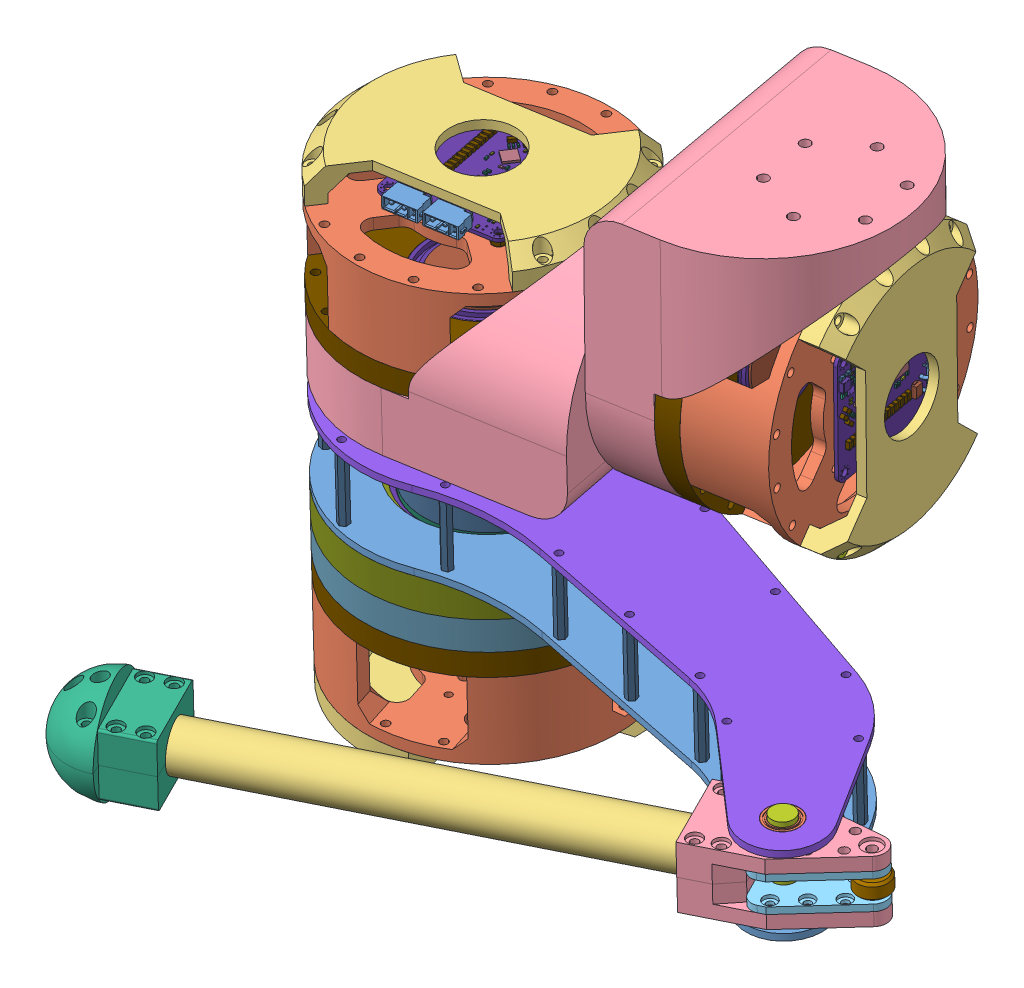
SolidWorks assembly leg, configuration Default. Lengths in mm. (continued)
Components (placement in the parent): (continued)
- Cycloidal _v3-1: Cycloidal _v3 [Default] at (95.6254 359.4899 346.7984) x (0.586151 0.024345 -0.809836) z (-0.810184 0.024334 -0.585671) size (173.36 87.57 173.15) (continued)
  - m13_bearing-34: m13_bearing [Default] at (13.4541 98.1947 126.1847) x (0.227678 0.000091 0.973736) z (0.973736 0.000388 -0.227678) size (13 16 13) (continued)
    - radial ball bearing_68_iso-1: radial ball bearing_68_iso [ISO 15 RBB - 286 - 10,SI,NC,10_68] at (8.4921 16.0508 14.8914) x (0 1 0) z (0 0 1) size (5 13 13)
    - radial ball bearing_68_iso-2: radial ball bearing_68_iso [ISO 15 RBB - 286 - 10,SI,NC,10_68] at (8.4921 11.0508 14.8914) x (0 1 0) z (0 0 1) size (5 13 13)
  - m13_bearing-35: m13_bearing [Default] at (-1.0662 98.1889 116.3132) x (0.227678 0.000091 0.973736) z (0.973736 0.000388 -0.227678) size (13 16 13)
    - m6-1: m6 [Default] at (8.4921 2.5508 14.8914) size (6 16 6)
    - radial ball bearing_68_iso-1: radial ball bearing_68_iso [ISO 15 RBB - 286 - 10,SI,NC,10_68] at (8.4921 16.0508 14.8914) x (0 1 0) z (0 0 1) size (5 13 13)
    - radial ball bearing_68_iso-2: radial ball bearing_68_iso [ISO 15 RBB - 286 - 10,SI,NC,10_68] at (8.4921 11.0508 14.8914) x (0 1 0) z (0 0 1) size (5 13 13)
  - m13_bearing-36: m13_bearing [Default] at (-10.7036 98.185 101.6364) x (0.227678 0.000091 0.973736) z (0.973736 0.000388 -0.227678) size (13 16 13)
    - m6-1: m6 [Default] at (8.4921 2.5508 14.8914) size (6 16 6)
    - radial ball bearing_68_iso-1: radial ball bearing_68_iso [ISO 15 RBB - 286 - 10,SI,NC,10_68] at (8.4921 16.0508 14.8914) x (0 1 0) z (0 0 1) size (5 13 13)
    - radial ball bearing_68_iso-2: radial ball bearing_68_iso [ISO 15 RBB - 286 - 10,SI,NC,10_68] at (8.4921 11.0508 14.8914) x (0 1 0) z (0 0 1) size (5 13 13)
  - m13_bearing-1: m13_bearing [Default] at (-0.4494 98.1891 62.778) x (0.736525 0.000294 0.676411) z (0.676411 0.00027 -0.736525) size (13 16 13)
    - m6-1: m6 [Default] at (8.4921 2.5508 14.8914) size (6 16 6)
    - radial ball bearing_68_iso-1: radial ball bearing_68_iso [ISO 15 RBB - 286 - 10,SI,NC,10_68] at (8.4921 16.0508 14.8914) x (0 1 0) z (0 0 1) size (5 13 13)
    - radial ball bearing_68_iso-2: radial ball bearing_68_iso [ISO 15 RBB - 286 - 10,SI,NC,10_68] at (8.4921 11.0508 14.8914) x (0 1 0) z (0 0 1) size (5 13 13)
  - m13_bearing-2: m13_bearing [Default] at (48.5236 98.2087 124.7001) x (0.120271 0.000048 0.992741) z (0.992741 0.000396 -0.120271) size (13 16 13)
    - m6-1: m6 [Default] at (8.4921 2.5508 14.8914) size (6 16 6)
    - radial ball bearing_68_iso-1: radial ball bearing_68_iso [ISO 15 RBB - 286 - 10,SI,NC,10_68] at (8.4921 16.0508 14.8914) x (0 1 0) z (0 0 1) size (5 13 13)
    - radial ball bearing_68_iso-2: radial ball bearing_68_iso [ISO 15 RBB - 286 - 10,SI,NC,10_68] at (8.4921 11.0508 14.8914) x (0 1 0) z (0 0 1) size (5 13 13)
  - m13_bearing-3: m13_bearing [Default] at (32.5019 98.2023 52.3604) x (0.833889 0.000333 0.551933) z (0.551932 0.00022 -0.833889) size (13 16 13)
    - m6-1: m6 [Default] at (8.4921 2.5508 14.8914) size (6 16 6)
    - radial ball bearing_68_iso-1: radial ball bearing_68_iso [ISO 15 RBB - 286 - 10,SI,NC,10_68] at (8.4921 16.0508 14.8914) x (0 1 0) z (0 0 1) size (5 13 13)
    - radial ball bearing_68_iso-2: radial ball bearing_68_iso [ISO 15 RBB - 286 - 10,SI,NC,10_68] at (8.4921 11.0508 14.8914) x (0 1 0) z (0 0 1) size (5 13 13)
  - m13_bearing-4: m13_bearing [Default] at (77.3632 98.2202 81.8307) x (0.022268 0.000009 0.999752) z (0.999752 0.000399 -0.022268) size (13 16 13)
    - m6-1: m6 [Default] at (8.4921 2.5508 14.8914) size (6 16 6)
    - radial ball bearing_68_iso-1: radial ball bearing_68_iso [ISO 15 RBB - 286 - 10,SI,NC,10_68] at (8.4921 16.0508 14.8914) x (0 1 0) z (0 0 1) size (5 13 13)
    - radial ball bearing_68_iso-2: radial ball bearing_68_iso [ISO 15 RBB - 286 - 10,SI,NC,10_68] at (8.4921 11.0508 14.8914) x (0 1 0) z (0 0 1) size (5 13 13)
  - m13_bearing-5: m13_bearing [Default] at (73.5091 98.2186 99.5852) x (0.059133 0.000024 0.99825) z (0.99825 0.000398 -0.059133) size (13 16 13)
    - m6-1: m6 [Default] at (8.4921 2.5508 14.8914) size (6 16 6)
    - radial ball bearing_68_iso-1: radial ball bearing_68_iso [ISO 15 RBB - 286 - 10,SI,NC,10_68] at (8.4921 16.0508 14.8914) x (0 1 0) z (0 0 1) size (5 13 13)
    - radial ball bearing_68_iso-2: radial ball bearing_68_iso [ISO 15 RBB - 286 - 10,SI,NC,10_68] at (8.4921 11.0508 14.8914) x (0 1 0) z (0 0 1) size (5 13 13)
  - m13_bearing-6: m13_bearing [Default] at (13.4333 98.1947 47.0643) x (0.451561 0.00018 0.89224) z (0.89224 0.000356 -0.451561) size (13 16 13)
    - m6-1: m6 [Default] at (8.4921 2.5508 14.8914) size (6 16 6)
    - radial ball bearing_68_iso-1: radial ball bearing_68_iso [ISO 15 RBB - 286 - 10,SI,NC,10_68] at (8.4921 16.0508 14.8914) x (0 1 0) z (0 0 1) size (5 13 13)
    - radial ball bearing_68_iso-2: radial ball bearing_68_iso [ISO 15 RBB - 286 - 10,SI,NC,10_68] at (8.4921 11.0508 14.8914) x (0 1 0) z (0 0 1) size (5 13 13)
  - m13_bearing-7: m13_bearing [Default] at (57.1526 98.2121 32.9496) x (-0.545813 -0.000218 0.837907) z (0.837907 0.000334 0.545813) size (13 16 13)
    - m6-1: m6 [Default] at (8.4921 2.5508 14.8914) size (6 16 6)
    - radial ball bearing_68_iso-1: radial ball bearing_68_iso [ISO 15 RBB - 286 - 10,SI,NC,10_68] at (8.4921 16.0508 14.8914) x (0 1 0) z (0 0 1) size (5 13 13)
    - radial ball bearing_68_iso-2: radial ball bearing_68_iso [ISO 15 RBB - 286 - 10,SI,NC,10_68] at (8.4921 11.0508 14.8914) x (0 1 0) z (0 0 1) size (5 13 13)
  - m13_bearing-8: m13_bearing [Default] at (73.1034 98.2185 66.7178) x (0.158553 0.000063 0.98735) z (0.98735 0.000394 -0.158553) size (13 16 13)
    - m6-1: m6 [Default] at (8.4921 2.5508 14.8914) size (6 16 6)
    - radial ball bearing_68_iso-1: radial ball bearing_68_iso [ISO 15 RBB - 286 - 10,SI,NC,10_68] at (8.4921 16.0508 14.8914) x (0 1 0) z (0 0 1) size (5 13 13)
    - radial ball bearing_68_iso-2: radial ball bearing_68_iso [ISO 15 RBB - 286 - 10,SI,NC,10_68] at (8.4921 11.0508 14.8914) x (0 1 0) z (0 0 1) size (5 13 13)
  - m13_bearing-9: m13_bearing [Default] at (74.5316 98.219 41.6624) x (-0.687134 -0.000274 0.72653) z (0.72653 0.00029 0.687134) size (13 16 13)
    - m6-1: m6 [Default] at (8.4921 2.5508 14.8914) size (6 16 6)
    - radial ball bearing_68_iso-1: radial ball bearing_68_iso [ISO 15 RBB - 286 - 10,SI,NC,10_68] at (8.4921 16.0508 14.8914) x (0 1 0) z (0 0 1) size (5 13 13)
    - radial ball bearing_68_iso-2: radial ball bearing_68_iso [ISO 15 RBB - 286 - 10,SI,NC,10_68] at (8.4921 11.0508 14.8914) x (0 1 0) z (0 0 1) size (5 13 13)
  - m13_bearing-11: m13_bearing [Default] at (30.0113 98.2013 136.2104) x (0.57351 0.000229 0.819198) z (0.819198 0.000327 -0.57351) size (13 16 13)
    - m6-1: m6 [Default] at (8.4921 2.5508 14.8914) size (6 16 6)
    - radial ball bearing_68_iso-1: radial ball bearing_68_iso [ISO 15 RBB - 286 - 10,SI,NC,10_68] at (8.4921 16.0508 14.8914) x (0 1 0) z (0 0 1) size (5 13 13)
    - radial ball bearing_68_iso-2: radial ball bearing_68_iso [ISO 15 RBB - 286 - 10,SI,NC,10_68] at (8.4921 11.0508 14.8914) x (0 1 0) z (0 0 1) size (5 13 13)
  - m13_bearing-12: m13_bearing [Default] at (62.5932 98.2143 116.7506) x (0.22335 0.000089 0.974738) z (0.974738 0.000389 -0.22335) size (13 16 13)
    - m6-1: m6 [Default] at (8.4921 2.5508 14.8914) size (6 16 6)
    - radial ball bearing_68_iso-1: radial ball bearing_68_iso [ISO 15 RBB - 286 - 10,SI,NC,10_68] at (8.4921 16.0508 14.8914) x (0 1 0) z (0 0 1) size (5 13 13)
    - radial ball bearing_68_iso-2: radial ball bearing_68_iso [ISO 15 RBB - 286 - 10,SI,NC,10_68] at (8.4921 11.0508 14.8914) x (0 1 0) z (0 0 1) size (5 13 13)
  - M3x4x4.2_brass_insert-22: M3x4x4.2_brass_insert [Default] at (43.4837 68.6558 90.1203) x (0.984609 0.000393 -0.174769) z (0.174769 0.00007 0.984609) size (4 4 4)
  - M3x4x4.2_brass_insert-23: M3x4x4.2_brass_insert [Default] at (51.4229 68.659 89.1361) x (0.984609 0.000393 -0.174769) z (0.174769 0.00007 0.984609) size (4 4 4)
  - radial ball bearing_68_iso-44: radial ball bearing_68_iso [ISO 15 RBB - 1715 - 26,SI,NC,26_68] at (47.2636 81.6573 88.1396) x (0.000399 -1 0) z (0.171535 0.000068 0.985178) size (4 21 21)
  - radial ball bearing_68_iso-45: radial ball bearing_68_iso [ISO 15 RBB - 1715 - 26,SI,NC,26_68] at (47.4429 94.6574 89.6282) x (0.000399 -1 0) z (0.819169 0.000327 0.573552) size (4 21 21)
  - radial ball bearing_68_iso-46: radial ball bearing_68_iso [ISO 15 RBB - 1715 - 26,SI,NC,26_68] at (47.6295 89.6575 91.1168) x (-0.000399 1 0) z (0 0 1) size (4 21 21)
  - foc-motor-controller.step-1: foc-motor-controller.step [Default] at (47.4677 32.6574 89.6282) x (0.701413 0.00028 0.712755) z (0.000399 -1 0) size (57.23 50 8.13)
    - RTA0040B.step-1: RTA0040B.step [Default] at (12.5014 -1.6986 1.595) x (-0.707107 -0.707107 0) z (0 0 1) size (6 6 1)
      - FRAME.step-1: FRAME.step [Default] x (1 0 0) z (0 -1 0) size (6 0.2 6)
        - SOLID.step-1: SOLID.step [Default] at origin size (0.4 0.2 0.22)
        - SOLID-0.step-1: SOLID-0.step [Default] at origin size (0.4 0.2 0.22)
        - SOLID-1.step-1: SOLID-1.step [Default] at origin size (0.4 0.2 0.22)
        - SOLID-2.step-1: SOLID-2.step [Default] at origin size (0.4 0.2 0.22)
        - SOLID-3.step-1: SOLID-3.step [Default] at origin size (0.4 0.2 0.22)
        - SOLID-4.step-1: SOLID-4.step [Default] at origin size (0.4 0.2 0.22)
        - SOLID-5.step-1: SOLID-5.step [Default] at origin size (0.4 0.2 0.22)
        - SOLID-6.step-1: SOLID-6.step [Default] at origin size (0.4 0.2 0.22)
        - SOLID-7.step-1: SOLID-7.step [Default] at origin size (0.4 0.2 0.22)
        - SOLID-8.step-1: SOLID-8.step [Default] at origin size (0.4 0.2 0.22)
        - SOLID-9.step-1: SOLID-9.step [Default] at origin size (0.22 0.2 0.4)
        - SOLID-10.step-1: SOLID-10.step [Default] at origin size (0.22 0.2 0.4)
        - SOLID-11.step-1: SOLID-11.step [Default] at origin size (0.22 0.2 0.4)
        - SOLID-12.step-1: SOLID-12.step [Default] at origin size (0.22 0.2 0.4)
        - SOLID-13.step-1: SOLID-13.step [Default] at origin size (0.22 0.2 0.4)
        - SOLID-14.step-1: SOLID-14.step [Default] at origin size (0.22 0.2 0.4)
        - SOLID-15.step-1: SOLID-15.step [Default] at origin size (0.22 0.2 0.4)
        - SOLID-16.step-1: SOLID-16.step [Default] at origin size (0.22 0.2 0.4)
        - SOLID-17.step-1: SOLID-17.step [Default] at origin size (4.15 0.2 4.15)
        - SOLID-18.step-1: SOLID-18.step [Default] at origin size (0.28 0.1 0.28)
        - SOLID-19.step-1: SOLID-19.step [Default] at origin size (0.28 0.1 0.28)
        - SOLID-20.step-1: SOLID-20.step [Default] at origin size (0.28 0.1 0.28)
        - SOLID-21.step-1: SOLID-21.step [Default] at origin size (0.28 0.1 0.28)
        - SOLID-22.step-1: SOLID-22.step [Default] at origin size (0.4 0.2 0.22)
        - SOLID-23.step-1: SOLID-23.step [Default] at origin size (0.4 0.2 0.22)
        - SOLID-24.step-1: SOLID-24.step [Default] at origin size (0.4 0.2 0.22)
        - SOLID-25.step-1: SOLID-25.step [Default] at origin size (0.4 0.2 0.22)
        - SOLID-26.step-1: SOLID-26.step [Default] at origin size (0.4 0.2 0.22)
        - SOLID-27.step-1: SOLID-27.step [Default] at origin size (0.4 0.2 0.22)
        - SOLID-28.step-1: SOLID-28.step [Default] at origin size (0.4 0.2 0.22)
        - SOLID-29.step-1: SOLID-29.step [Default] at origin size (0.4 0.2 0.22)
        - SOLID-30.step-1: SOLID-30.step [Default] at origin size (0.4 0.2 0.22)
        - SOLID-31.step-1: SOLID-31.step [Default] at origin size (0.4 0.2 0.22)
        - SOLID-32.step-1: SOLID-32.step [Default] at origin size (0.22 0.2 0.4)
        - SOLID-33.step-1: SOLID-33.step [Default] at origin size (0.22 0.2 0.4)
        - SOLID-34.step-1: SOLID-34.step [Default] at origin size (0.22 0.2 0.4)
        - SOLID-35.step-1: SOLID-35.step [Default] at origin size (0.22 0.2 0.4)
        - SOLID-36.step-1: SOLID-36.step [Default] at origin size (0.22 0.2 0.4)
        - SOLID-37.step-1: SOLID-37.step [Default] at origin size (0.22 0.2 0.4)
        - SOLID-38.step-1: SOLID-38.step [Default] at origin size (0.22 0.2 0.4)
        - SOLID-39.step-1: SOLID-39.step [Default] at origin size (0.22 0.2 0.4)
        - SOLID-40.step-1: SOLID-40.step [Default] at origin size (0.22 0.2 0.4)
        - SOLID-41.step-1: SOLID-41.step [Default] at origin size (0.22 0.2 0.4)
        - SOLID-42.step-1: SOLID-42.step [Default] at origin size (0.22 0.2 0.4)
        - SOLID-43.step-1: SOLID-43.step [Default] at origin size (0.22 0.2 0.4)
      - BODY.step-1: BODY.step [Default] at (0 0 0.025) x (1 0 0) z (0 -1 0) size (6 0.97 6)
    - Resonator_SMD_Murata_CSTxExxV-3Pin_3.0x1.1mm.step-1: Resonator_SMD_Murata_CSTxExxV-3Pin_3.0x1.1mm.step [Default] at (1.8 -7 1.595) x (0 1 0) z (0 0 1) size (3.2 1.35 0.9)
    - C_0603_1608Metric.step-1: C_0603_1608Metric.step [Default] at (6.2 -16.8 1.595) x (0 -1 0) z (0 0 1) size (1.6 0.8 0.8)
    - R_0603_1608Metric.step-1: R_0603_1608Metric.step [Default] at (11.8 -7.375 1.595) x (0 1 0) z (0 0 1) size (1.6 0.8 0.45)
    - R_0603_1608Metric.step-2: R_0603_1608Metric.step [Default] at (13.8 -16.8 1.595) x (0 1 0) z (0 0 1) size (1.6 0.8 0.45)
    - R_0603_1608Metric.step-3: R_0603_1608Metric.step [Default] at (18.1 -5.36 1.595) size (1.6 0.8 0.45)
    - C_0603_1608Metric.step-2: C_0603_1608Metric.step [Default] at (2.6 -0.5 1.595) x (0 -1 0) z (0 0 1) size (1.6 0.8 0.8)
    - R_0603_1608Metric.step-4: R_0603_1608Metric.step [Default] at (14.6 -11.3 1.595) x (0 1 0) z (0 0 1) size (1.6 0.8 0.45)
    - L_APV_ANR4020.step-1: L_APV_ANR4020.step [Default] at (22.3 -13.7 1.595) x (0 -1 0) z (0 0 1) size (4.02 4 2)
    - C_0603_1608Metric.step-3: C_0603_1608Metric.step [Default] at (0.3 -12.6 1.595) x (-1 0 0) z (0 0 1) size (1.6 0.8 0.8)
    - C_1206_3216Metric.step-1: C_1206_3216Metric.step [Default] at (15.7 11 1.595) x (0 1 0) z (0 0 1) size (3.2 1.6 1.6)
    - C_0603_1608Metric.step-4: C_0603_1608Metric.step [Default] at (0.3 -9.6 1.595) size (1.6 0.8 0.8)
    - R_0603_1608Metric.step-5: R_0603_1608Metric.step [Default] at (12.3 -16.8 1.595) x (0 1 0) z (0 0 1) size (1.6 0.8 0.45)
    - C_0603_1608Metric.step-5: C_0603_1608Metric.step [Default] at (-0.3 -16.6 1.595) x (0 1 0) z (0 0 1) size (1.6 0.8 0.8)
    - R_0603_1608Metric.step-6: R_0603_1608Metric.step [Default] at (10.9 4.1 1.595) size (1.6 0.8 0.45)
    - C_1206_3216Metric.step-2: C_1206_3216Metric.step [Default] at (6.3 11 1.595) x (0 1 0) z (0 0 1) size (3.2 1.6 1.6)
    - XT30PW_2_2_-M.G.B.step-1: XT30PW_2_2_-M.G.B.step [Default] at (-20.5 9.5 1.595) x (0 -1 0) z (-1 0 0) size (15.5 7.1 12.53)
    - R_0603_1608Metric.step-7: R_0603_1608Metric.step [Default] at (0.3 -11.1 1.595) size (1.6 0.8 0.45)
    - C_0603_1608Metric.step-6: C_0603_1608Metric.step [Default] at (19 -0.4 1.595) x (-0.707107 -0.707107 0) z (0 0 1) size (1.6 0.8 0.8)
    - C_1206_3216Metric.step-3: C_1206_3216Metric.step [Default] at (13.3 11 1.595) x (0 1 0) z (0 0 1) size (3.2 1.6 1.6)
    - R_0603_1608Metric.step-8: R_0603_1608Metric.step [Default] at (10.2 -7.375 1.595) x (0 -1 0) z (0 0 1) size (1.6 0.8 0.45)
    - JST_GH_SM08B-GHS-TB_1x08-1MP_P1.25mm_Horizontal.step-1: JST_GH_SM08B-GHS-TB_1x08-1MP_P1.25mm_Horizontal.step [Default] at (10 -22 1.595) size (13.25 4.95 4.25)
    - C_1206_3216Metric.step-4: C_1206_3216Metric.step [Default] at (-12.3 11 1.595) x (0 1 0) z (0 0 1) size (3.2 1.6 1.6)
    - JST_GH_SM06B-GHS-TB_1x06-1MP_P1.25mm_Horizontal.step-1: JST_GH_SM06B-GHS-TB_1x06-1MP_P1.25mm_Horizontal.step [Default] at (-4.3 -22 1.595) size (10.75 4.95 4.25)
    - C_0603_1608Metric.step-7: C_0603_1608Metric.step [Default] at (7.3 -4.5 1.595) x (-1 0 0) z (0 0 1) size (1.6 0.8 0.8)
    - R_0603_1608Metric.step-9: R_0603_1608Metric.step [Default] at (18.1 -3.86 1.595) x (-1 0 0) z (0 0 1) size (1.6 0.8 0.45)
    - C_1206_3216Metric.step-5: C_1206_3216Metric.step [Default] at (22.6794 -1.2206 1.595) x (0.707107 -0.707107 0) z (0 0 1) size (3.2 1.6 1.6)
    - R_Array_Convex_4x0402.step-1: R_Array_Convex_4x0402.step [Default] at (6.8 -2.5 1.595) size (1 2 0.35)
    - R_0603_1608Metric.step-10: R_0603_1608Metric.step [Default] at (7.7 -16.8 1.595) x (0 -1 0) z (0 0 1) size (1.6 0.8 0.45)
    - C_1206_3216Metric.step-6: C_1206_3216Metric.step [Default] at (8.7 11 1.595) x (0 1 0) z (0 0 1) size (3.2 1.6 1.6)
    - C_0603_1608Metric.step-8: C_0603_1608Metric.step [Default] at (16.1 -11.3 1.595) x (0 1 0) z (0 0 1) size (1.6 0.8 0.8)
    - SOT-23-5.step-1: SOT-23-5.step [Default] at (-3.1 -16.6 1.595) x (-1 0 0) z (0 0 1) size (2.8 2.9 1.55)
    - C_0603_1608Metric.step-9: C_0603_1608Metric.step [Default] at (17.8 -13.6 1.595) size (1.6 0.8 0.8)
    - R_0603_1608Metric.step-11: R_0603_1608Metric.step [Default] at (-11.5 -20.3875 1.595) x (0 -1 0) z (0 0 1) size (1.6 0.8 0.45)
    - C_0603_1608Metric.step-10: C_0603_1608Metric.step [Default] at (-12.4 2.3 1.595) x (0 1 0) z (0 0 1) size (1.6 0.8 0.8)
    - C_1206_3216Metric.step-7: C_1206_3216Metric.step [Default] at (18 11 1.595) x (0 1 0) z (0 0 1) size (3.2 1.6 1.6)
    - R_0603_1608Metric.step-12: R_0603_1608Metric.step [Default] at (-10.8105 -14.9971 1.595) x (-1 0 0) z (0 0 1) size (1.6 0.8 0.45)
    - C_0603_1608Metric.step-11: C_0603_1608Metric.step [Default] at (-13.8 -9.4 1.595) x (-1 0 0) z (0 0 1) size (1.6 0.8 0.8)
    - R_0603_1608Metric.step-13: R_0603_1608Metric.step [Default] at (-23.15 -14.5 1.595) x (-1 0 0) z (0 0 1) size (1.6 0.8 0.45)
    - C_0603_1608Metric.step-12: C_0603_1608Metric.step [Default] at (1.1 -0.2 1.595) x (0 1 0) z (0 0 1) size (1.6 0.8 0.8)
    - D_0805_2012Metric.step-1: D_0805_2012Metric.step [Default] at (22.9 -9.6 1.595) x (0 1 0) z (0 0 1) size (2 1.27 0.8)
    - C_0603_1608Metric.step-13: C_0603_1608Metric.step [Default] at (-7.8 3.775 1.595) x (0 -1 0) z (0 0 1) size (1.6 0.8 0.8)
    - R_0603_1608Metric.step-14: R_0603_1608Metric.step [Default] at (-6.4 -12.825 1.595) x (0 1 0) z (0 0 1) size (1.6 0.8 0.45)
    - L_0603_1608Metric.step-1: L_0603_1608Metric.step [Default] at (-10.1 3 1.595) size (1.6 0.8 0.8)
    - C_0603_1608Metric.step-14: C_0603_1608Metric.step [Default] at (17.9 0.7 1.595) x (-0.707107 -0.707107 0) z (0 0 1) size (1.6 0.8 0.8)
    - HVSSOP-10.step-1: HVSSOP-10.step [Default] at (18.6 -9.6 1.595) x (0 -1 0) z (-1 0 0) size (4.9 1.1 3)
    - C_0603_1608Metric.step-15: C_0603_1608Metric.step [Default] at (7.9 4.1 1.595) x (-1 0 0) z (0 0 1) size (1.6 0.8 0.8)
    - C_0603_1608Metric.step-16: C_0603_1608Metric.step [Default] at (21.1 -9.6 1.595) x (0 -1 0) z (0 0 1) size (1.6 0.8 0.8)
    - R_0603_1608Metric.step-15: R_0603_1608Metric.step [Default] at (-10.8105 -11.9971 1.595) x (-1 0 0) z (0 0 1) size (1.6 0.8 0.45)
    - R_0603_1608Metric.step-16: R_0603_1608Metric.step [Default] at (-18.2 -17.4 1.595) size (1.6 0.8 0.45)
    - C_1206_3216Metric.step-8: C_1206_3216Metric.step [Default] at (-3 11 1.595) x (0 1 0) z (0 0 1) size (3.2 1.6 1.6)
    - R_0603_1608Metric.step-17: R_0603_1608Metric.step [Default] at (-16.9 -20.4 1.595) x (0 -1 0) z (0 0 1) size (1.6 0.8 0.45)
    - R_0603_1608Metric.step-18: R_0603_1608Metric.step [Default] at (-13.3 -20.3875 1.595) x (0 -1 0) z (0 0 1) size (1.6 0.8 0.45)
    - R_0603_1608Metric.step-19: R_0603_1608Metric.step [Default] at (-15.1 -20.3875 1.595) x (0 -1 0) z (0 0 1) size (1.6 0.8 0.45)
    - C_0603_1608Metric.step-17: C_0603_1608Metric.step [Default] at (15.5 -14.4 1.595) x (0 -1 0) z (0 0 1) size (1.6 0.8 0.8)
    - LED_0603_1608Metric.step-1: LED_0603_1608Metric.step [Default] at (-11.5 -23.3875 1.595) x (0 1 0) z (0 0 1) size (1.6 0.8 1.1)
    - C_0805_2012Metric.step-1: C_0805_2012Metric.step [Default] at (19.95 -17 1.595) size (2 1.25 1.25)
    - D_SMB.step-1: D_SMB.step [Default] at (-16.5 11.208 1.595) x (0 -1 0) z (0 0 1) size (5.3 3.55 2.15)
    - C_1206_3216Metric.step-9: C_1206_3216Metric.step [Default] at (-5.3 11 1.595) x (0 1 0) z (0 0 1) size (3.2 1.6 1.6)
    - XT30PW_2_2_-M.G.B.step-2: XT30PW_2_2_-M.G.B.step [Default] at (-20.5 -6.5 1.595) x (0 -1 0) z (-1 0 0) size (15.5 7.1 12.53)
    - C_1206_3216Metric.step-10: C_1206_3216Metric.step [Default] at (1.7 11 1.595) x (0 1 0) z (0 0 1) size (3.2 1.6 1.6)
    - C_1206_3216Metric.step-11: C_1206_3216Metric.step [Default] at (11 11 1.595) x (0 1 0) z (0 0 1) size (3.2 1.6 1.6)
    - C_0603_1608Metric.step-18: C_0603_1608Metric.step [Default] at (-6.3 3.775 1.595) x (0 -1 0) z (0 0 1) size (1.6 0.8 0.8)
    - C_0603_1608Metric.step-19: C_0603_1608Metric.step [Default] at (16.8686 1.7314 1.595) x (0.707107 0.707107 0) z (0 0 1) size (1.6 0.8 0.8)
    - C_0603_1608Metric.step-20: C_0603_1608Metric.step [Default] at (-15.0105 -11.1 1.595) size (1.6 0.8 0.8)
    - C_1206_3216Metric.step-12: C_1206_3216Metric.step [Default] at (-7.7 11 1.595) x (0 1 0) z (0 0 1) size (3.2 1.6 1.6)
    - C_0603_1608Metric.step-21: C_0603_1608Metric.step [Default] at (-18.2 -15.8 1.595) size (1.6 0.8 0.8)
    - C_0603_1608Metric.step-22: C_0603_1608Metric.step [Default] at (-2.1 -11.3 1.595) x (0 -1 0) z (0 0 1) size (1.6 0.8 0.8)
    - C_0603_1608Metric.step-23: C_0603_1608Metric.step [Default] at (-10.8105 -13.4971 1.595) size (1.6 0.8 0.8)
    - C_1206_3216Metric.step-13: C_1206_3216Metric.step [Default] at (4 11 1.595) x (0 1 0) z (0 0 1) size (3.2 1.6 1.6)
    - R_0603_1608Metric.step-20: R_0603_1608Metric.step [Default] at (16 -17.8 1.595) x (0 1 0) z (0 0 1) size (1.6 0.8 0.45)
    - Texas_S-PVSON-N8.step-1: Texas_S-PVSON-N8.step [Default] at (-14.4105 -13.7 1.595) x (-1 0 0) z (0 0 1) size (3 2.98 0.92)
    - C_1206_3216Metric.step-14: C_1206_3216Metric.step [Default] at (21 -2.9 1.595) x (0.707107 -0.707107 0) z (0 0 1) size (3.2 1.6 1.6)
    - C_0603_1608Metric.step-24: C_0603_1608Metric.step [Default] at (-5.9 -16.6 1.595) x (0 1 0) z (0 0 1) size (1.6 0.8 0.8)
    - C_0603_1608Metric.step-25: C_0603_1608Metric.step [Default] at (-3.1 -14.1 1.595) size (1.6 0.8 0.8)
    - R_0603_1608Metric.step-21: R_0603_1608Metric.step [Default] at (7.2 -7.375 1.595) x (0 -1 0) z (0 0 1) size (1.6 0.8 0.45)
    - C_1206_3216Metric.step-15: C_1206_3216Metric.step [Default] at (-0.7 11 1.595) x (0 1 0) z (0 0 1) size (3.2 1.6 1.6)
    - LQFP-64_10x10mm_P0.5mm.step-1: LQFP-64_10x10mm_P0.5mm.step [Default] at (-7 -4.5 1.595) x (-1 0 0) z (0 0 1) size (12 12 1.5)
    - C_0805_2012Metric.step-2: C_0805_2012Metric.step [Default] at (23.35 -17 1.595) x (-1 0 0) z (0 0 1) size (2 1.25 1.25)
    - C_0603_1608Metric.step-26: C_0603_1608Metric.step [Default] at (10.8 -16.8 1.595) x (0 -1 0) z (0 0 1) size (1.6 0.8 0.8)
    - R_0603_1608Metric.step-22: R_0603_1608Metric.step [Default] at (17.5 -17.8 1.595) x (0 -1 0) z (0 0 1) size (1.6 0.8 0.45)
    - C_1206_3216Metric.step-16: C_1206_3216Metric.step [Default] at (20.3 11 1.595) x (0 1 0) z (0 0 1) size (3.2 1.6 1.6)
    - R_0603_1608Metric.step-23: R_0603_1608Metric.step [Default] at (9.2 -16.8 1.595) x (0 -1 0) z (0 0 1) size (1.6 0.8 0.45)
    - C_1206_3216Metric.step-17: C_1206_3216Metric.step [Default] at (-10 11 1.595) x (0 1 0) z (0 0 1) size (3.2 1.6 1.6)
    - R_0603_1608Metric.step-24: R_0603_1608Metric.step [Default] at (17.8 -15.2 1.595) size (1.6 0.8 0.45)
    - C_1206_3216Metric.step-18: C_1206_3216Metric.step [Default] at (19.9 2.6 1.595) x (-0.707107 0.707107 0) z (0 0 1) size (3.2 1.6 1.6)
    - C_0603_1608Metric.step-27: C_0603_1608Metric.step [Default] at (13.4 -7.375 1.595) x (0 -1 0) z (0 0 1) size (1.6 0.8 0.8)
    - R_0603_1608Metric.step-25: R_0603_1608Metric.step [Default] at (8.7 -7.375 1.595) x (0 -1 0) z (0 0 1) size (1.6 0.8 0.45)
    - PQFN-8-EP_6x5mm_P1.27mm_Generic.step-1: PQFN-8-EP_6x5mm_P1.27mm_Generic.step [Default] at (4.9 14.4 -0.085) x (0 1 0) z (0 0 -1) size (6.15 5.15 1.09)
    - C_0805_2012Metric.step-3: C_0805_2012Metric.step [Default] at (-3 8.9 -0.085) x (0 1 0) z (0 0 -1) size (2 1.25 1.25)
    - C_0603_1608Metric.step-28: C_0603_1608Metric.step [Default] at (1.5 -4.3 -0.085) x (0 1 0) z (0 0 -1) size (1.6 0.8 0.8)
    - R_2512_6332Metric.step-1: R_2512_6332Metric.step [Default] at (2.1 8.6 -0.085) x (-1 0 0) z (0 0 -1) size (6.3 3.2 0.6)
    - C_0805_2012Metric.step-4: C_0805_2012Metric.step [Default] at (18.8 8.9 -0.085) x (0 1 0) z (0 0 -1) size (2 1.25 1.25)
    - C_0805_2012Metric.step-5: C_0805_2012Metric.step [Default] at (-5.2 8.901 -0.085) x (0 1 0) z (0 0 -1) size (2 1.25 1.25)
    - PQFN-8-EP_6x5mm_P1.27mm_Generic.step-2: PQFN-8-EP_6x5mm_P1.27mm_Generic.step [Default] at (16.9 14.6 -0.085) x (0 -1 0) z (0 0 -1) size (6.15 5.15 1.09)
    - PQFN-8-EP_6x5mm_P1.27mm_Generic.step-3: PQFN-8-EP_6x5mm_P1.27mm_Generic.step [Default] at (-1.1 14.6 -0.085) x (0 -1 0) z (0 0 -1) size (6.15 5.15 1.09)
    - R_0603_1608Metric.step-26: R_0603_1608Metric.step [Default] at (8.2 8.8 -0.085) x (0 1 0) z (0 0 -1) size (1.6 0.8 0.45)
    - R_2512_6332Metric.step-2: R_2512_6332Metric.step [Default] at (-10.3 8.601 -0.085) x (1 0 0) z (0 0 -1) size (6.3 3.2 0.6)
    - TSSOP-16_4.4x5mm_P0.65mm.step-1: TSSOP-16_4.4x5mm_P0.65mm.step [Default] at (0 0 -0.085) x (-1 0 0) z (0 0 -1) size (6.4 5 1.1)
    - C_0603_1608Metric.step-29: C_0603_1608Metric.step [Default] at (0 -4.25 -0.085) x (0 1 0) z (0 0 -1) size (1.6 0.8 0.8)
    - PQFN-8-EP_6x5mm_P1.27mm_Generic.step-4: PQFN-8-EP_6x5mm_P1.27mm_Generic.step [Default] at (10.9 14.4 -0.085) x (0 1 0) z (0 0 -1) size (6.15 5.15 1.09)
    - R_2512_6332Metric.step-3: R_2512_6332Metric.step [Default] at (13.7 8.6 -0.085) x (1 0 0) z (0 0 -1) size (6.3 3.2 0.6)
    - PQFN-8-EP_6x5mm_P1.27mm_Generic.step-5: PQFN-8-EP_6x5mm_P1.27mm_Generic.step [Default] at (-13.1 14.401 -0.085) x (0 1 0) z (0 0 -1) size (6.15 5.15 1.09)
    - C_0603_1608Metric.step-30: C_0603_1608Metric.step [Default] at (-1.5 -4.3 -0.085) x (0 -1 0) z (0 0 -1) size (1.6 0.8 0.8)
    - PQFN-8-EP_6x5mm_P1.27mm_Generic.step-6: PQFN-8-EP_6x5mm_P1.27mm_Generic.step [Default] at (-7.1 14.601 -0.085) x (0 -1 0) z (0 0 -1) size (6.15 5.15 1.09)
    - foc-motor-controller_PCB.step-1: foc-motor-controller_PCB.step [Default] at origin size (50 50 1.51)
  - hex nut style 1 gradeab_iso-1: hex nut style 1 gradeab_iso [ISO - 4032 - M3 - W - N] at (47.7115 32.6575 59.2236) x (1 0.000399 0) z (0.000399 -1 0) size (5.5 6.35 2.4)
  - Cycloidal_Discs_8308-1: Cycloidal_Discs_8308 [Default] at (-11.9184 124.164 51.5043) x (0.028527 0.000011 0.999593) z (0.999593 0.000399 -0.028527) size (79.25 5 79.73)
    - Cycloidal_Discs-1: Cycloidal_Discs [Default] at (38.3081 39.5303 58.0959) size (79.25 5 79.73)
  - Cycloidal_Discs_8308-2: Cycloidal_Discs_8308 [Default] at (62.1667 47.133 159.1742) x (-0.931329 -0.000371 -0.364178) z (0.364178 0.000145 -0.931329) size (79.25 5 79.73)
    - Cycloidal_Discs-1: Cycloidal_Discs [Default] at (38.3081 39.5303 58.0959) size (79.25 5 79.73)
  - Motor_Cover_v2-2: Motor_Cover_v2 [Default] at (47.4667 35.0574 89.6282) x (0.999968 0.000399 0.00802) z (-0.00802 -0.000003 0.999968) size (115 34.6 115)
  - driver_cover-1: driver_cover [Default] at (47.4667 35.0574 89.6282) x (0.702656 0.00028 0.711529) z (0.711529 0.000284 -0.702656) size (81.32 15 115)
  - Cover_new-1: Cover_new [Default] at (47.4437 92.6574 89.6282) x (0.701413 0.00028 0.712755) z (-0.712755 -0.000284 0.701413) size (115 87.5 130)
  - Output_Shaft-2: Output_Shaft [Default] at (47.4437 92.6574 89.6282) x (0.572675 0.000228 0.819783) z (-0.819783 -0.000327 0.572675) size (70 14 70)
  - radial ball bearing_68_iso-47: radial ball bearing_68_iso [ISO 15 RBB - 289 - 14,SI,NC,14_68] at (61.9924 89.1632 109.081) x (0.000399 -1 0) z (-0.055662 -0.000022 0.99845) size (5 17 17)
  - radial ball bearing_68_iso-48: radial ball bearing_68_iso [ISO 15 RBB - 289 - 14,SI,NC,14_68] at (59.3269 82.1622 107.722) x (0.000399 -1 0) z (-0.055662 -0.000022 0.99845) size (5 17 17)
  - m4x14-1: m4x14 [Default] at (47.0925 68.4573 134.6267) x (0.999623 0.000399 0.027466) z (-0.027466 -0.000011 0.999623) size (8 15.2 8)
  - M3x20-1: M3x20 [Default] at (43.4726 96.3558 90.1203) x (-0.837193 -0.000334 -0.546908) z (-0.546908 -0.000218 0.837193) size (6 21.2 6)
  - M3x10-1: M3x10 [Default] at (36.5111 25.853 142.5044) x (0.424034 0.000169 -0.905646) z (0.905646 0.000361 0.424034) size (6 11.2 6)
  - m3x60-1: m3x60 [Default] at (17.1068 35.0453 134.2855) x (-0.837193 -0.000334 -0.546908) z (-0.546908 -0.000218 0.837193) size (5.3 63 5.3)
  - m6-1: m6 [Default] at (60.6129 98.6627 108.4832) x (-0.153131 -0.000061 0.988206) z (0.988206 0.000394 0.153131) size (6 16 6)
- Output_2-1: Output_2 [Default] at (50.2351 256.2315 252.2647) x (-0.122355 0.034106 -0.9919) z (-0.99247 0.001517 0.122478) size (60 8 60)
- Brass_m3-1: Brass_m3 [Default] at (3.4392 214.5993 278.2235) x (-0.332314 0.033638 -0.942569) z (0.943152 0.005831 -0.332311) size (4.62 30 4)
- Brass_m3-2: Brass_m3 [Default] at (-2.2595 216.0097 237.3127) x (0.431928 0.027909 -0.901476) z (0.90189 -0.019662 0.431517) size (4.62 30 4)
- Brass_m3-3: Brass_m3 [Default] at (22.6558 216.9783 204.3515) x (0.943152 0.005831 -0.332311) z (0.332314 -0.033638 0.942569) size (4.62 30 4)
- Brass_m3-4: Brass_m3 [Default] at (63.5902 216.9377 198.6481) x (0.90189 -0.019662 0.431517) z (-0.431928 -0.027909 0.901476) size (4.62 30 4)
- Brass_m3-5: Brass_m3 [Default] at (96.5648 215.9117 223.5434) x (0.332314 -0.033638 0.942569) z (-0.943152 -0.005831 0.332311) size (4.62 30 4)
- Brass_m3-7: Brass_m3 [Default] at (77.3482 213.5326 297.4154) x (-0.943152 -0.005831 0.332311) z (-0.332314 0.033638 -0.942569) size (4.62 30 4)
- Brass_m3-8: Brass_m3 [Default] at (36.4138 213.5733 303.1188) x (-0.90189 0.019662 -0.431517) z (0.431928 0.027909 -0.901476) size (4.62 30 4)
- Brass_m3-9: Brass_m3 [Default] at (231.0347 211.7498 324.406) x (-0.332314 0.033638 -0.942569) z (0.943152 0.005831 -0.332311) size (4.62 30 4)
- Brass_m3-10: Brass_m3 [Default] at (267.9904 212.2932 302.0366) x (-0.332314 0.033638 -0.942569) z (0.943152 0.005831 -0.332311) size (4.62 30 4)
- Brass_m3-11: Brass_m3 [Default] at (207.7434 212.262 313.1311) x (-0.3313 0.033645 -0.942925) z (0.943508 0.005795 -0.331299) size (4.62 30 4)
- Brass_m3-12: Brass_m3 [Default] at (241.1487 213.1591 280.8575) x (-0.332314 0.033638 -0.942569) z (0.943152 0.005831 -0.332311) size (4.62 30 4)
- Brass_m3-15: Brass_m3 [Default] at (193.6773 213.9572 265.1785) x (-0.332314 0.033638 -0.942569) z (0.943152 0.005831 -0.332311) size (4.62 30 4)
- Brass_m3-16: Brass_m3 [Default] at (146.206 214.7552 249.4995) x (-0.332314 0.033638 -0.942569) z (0.943152 0.005831 -0.332311) size (4.62 30 4)
- Brass_m3-17: Brass_m3 [Default] at (168.4593 212.7386 305.612) x (-0.3313 0.033645 -0.942925) z (0.943508 0.005795 -0.331299) size (4.62 30 4)
- Brass_m3-18: Brass_m3 [Default] at (129.1753 213.2152 298.0929) x (-0.3313 0.033645 -0.942925) z (0.943508 0.005795 -0.331299) size (4.62 30 4)
- Cycloidal _v3-2: Cycloidal _v3 [Default] at (218.9878 344.1312 127.6496) x (0.118839 0.702482 0.701709) z (0.116912 -0.711701 0.692685) size (173.36 87.57 173.15)
  - motor-X83008S.stp-1: motor-X83008S.stp [Default] at (3.9105 88.7742 94.1058) x (0.928336 0.00037 -0.371741) z (0.000399 -1 0) size (114.7 114.7 37.62) (hidden)
    - base.stp-1: base.stp [Default] at (42.0794 12.0269 46.7342) size (91.6 91.6 15.61)
    - stator.stp-1: stator.stp [Default] at (42.0794 12.0269 33.1342) x (0.08493 -0.996387 0) z (0 0 1) size (83 83 8)
    - coil.stp-1: coil.stp [Default] at (39.5332 41.8984 37.1342) x (0.996387 0.08493 0) z (-0.08493 0.996387 0) size (4.4 10.2 10.5)
    - coil.stp-2: coil.stp [Default] at (34.3848 41.0025 37.1342) x (0.966502 0.256661 0) z (-0.256661 0.966502 0) size (4.4 10.2 10.5)
    - coil.stp-3: coil.stp [Default] at (29.4701 39.2261 37.1342) x (0.90725 0.420593 0) z (-0.420593 0.90725 0) size (4.4 10.2 10.5)
    - coil.stp-4: coil.stp [Default] at (24.9386 36.6233 37.1342) x (0.820431 0.571745 0) z (-0.571745 0.820431 0) size (4.4 10.2 10.5)
    - coil.stp-5: coil.stp [Default] at (20.9279 33.2732 37.1342) x (0.708685 0.705525 0) z (-0.705525 0.708685 0) size (4.4 10.2 10.5)
    - coil.stp-6: coil.stp [Default] at (17.5599 29.2775 37.1342) x (0.575405 0.817869 0) z (-0.817869 0.575405 0) size (4.4 10.2 10.5)
    - coil.stp-7: coil.stp [Default] at (14.9368 24.7576 37.1342) x (0.424642 0.905361 0) z (-0.905361 0.424642 0) size (4.4 10.2 10.5)
    - coil.stp-8: coil.stp [Default] at (13.1385 19.8509 37.1342) x (0.260976 0.965345 0) z (-0.965345 0.260976 0) size (4.4 10.2 10.5)
    - coil.stp-9: coil.stp [Default] at (12.2196 14.7066 37.1342) x (0.089381 0.995998 0) z (-0.995998 0.089381 0) size (4.4 10.2 10.5)
    - coil.stp-10: coil.stp [Default] at (12.2079 9.4807 37.1342) x (-0.08493 0.996387 0) z (-0.996387 -0.08493 0) size (4.4 10.2 10.5)
    - coil.stp-11: coil.stp [Default] at (13.1039 4.3323 37.1342) x (-0.256661 0.966502 0) z (-0.966502 -0.256661 0) size (4.4 10.2 10.5)
    - coil.stp-12: coil.stp [Default] at (14.8802 -0.5824 37.1342) x (-0.420593 0.90725 0) z (-0.90725 -0.420593 0) size (4.4 10.2 10.5)
    - coil.stp-13: coil.stp [Default] at (17.483 -5.1139 37.1342) x (-0.571745 0.820431 0) z (-0.820431 -0.571745 0) size (4.4 10.2 10.5)
    - coil.stp-14: coil.stp [Default] at (20.8332 -9.1246 37.1342) x (-0.705525 0.708685 0) z (-0.708685 -0.705525 0) size (4.4 10.2 10.5)
    - coil.stp-15: coil.stp [Default] at (24.8289 -12.4926 37.1342) x (-0.817869 0.575405 0) z (-0.575405 -0.817869 0) size (4.4 10.2 10.5)
    - coil.stp-16: coil.stp [Default] at (29.3487 -15.1157 37.1342) x (-0.905361 0.424642 0) z (-0.424642 -0.905361 0) size (4.4 10.2 10.5)
    - coil.stp-17: coil.stp [Default] at (34.2554 -16.914 37.1342) x (-0.965345 0.260976 0) z (-0.260976 -0.965345 0) size (4.4 10.2 10.5)
    - coil.stp-18: coil.stp [Default] at (39.3998 -17.8329 37.1342) x (-0.995998 0.089381 0) z (-0.089381 -0.995998 0) size (4.4 10.2 10.5)
    - coil.stp-19: coil.stp [Default] at (44.6256 -17.8446 37.1342) x (-0.996387 -0.08493 0) z (0.08493 -0.996387 0) size (4.4 10.2 10.5)
    - coil.stp-20: coil.stp [Default] at (49.7741 -16.9486 37.1342) x (-0.966502 -0.256661 0) z (0.256661 -0.966502 0) size (4.4 10.2 10.5)
    - coil.stp-21: coil.stp [Default] at (54.6887 -15.1723 37.1342) x (-0.90725 -0.420593 0) z (0.420593 -0.90725 0) size (4.4 10.2 10.5)
    - coil.stp-22: coil.stp [Default] at (59.2202 -12.5695 37.1342) x (-0.820431 -0.571745 0) z (0.571745 -0.820431 0) size (4.4 10.2 10.5)
    - coil.stp-23: coil.stp [Default] at (63.2309 -9.2193 37.1342) x (-0.708685 -0.705525 0) z (0.705525 -0.708685 0) size (4.4 10.2 10.5)
    - coil.stp-24: coil.stp [Default] at (66.599 -5.2236 37.1342) x (-0.575405 -0.817869 0) z (0.817869 -0.575405 0) size (4.4 10.2 10.5)
    - coil.stp-25: coil.stp [Default] at (69.222 -0.7038 37.1342) x (-0.424642 -0.905361 0) z (0.905361 -0.424642 0) size (4.4 10.2 10.5)
    - coil.stp-26: coil.stp [Default] at (71.0203 4.2029 37.1342) x (-0.260976 -0.965345 0) z (0.965345 -0.260976 0) size (4.4 10.2 10.5)
    - coil.stp-27: coil.stp [Default] at (71.9392 9.3473 37.1342) x (-0.089381 -0.995998 0) z (0.995998 -0.089381 0) size (4.4 10.2 10.5)
    - coil.stp-28: coil.stp [Default] at (71.9509 14.5731 37.1342) x (0.08493 -0.996387 0) z (0.996387 0.08493 0) size (4.4 10.2 10.5)
    - coil.stp-29: coil.stp [Default] at (71.055 19.7216 37.1342) x (0.256661 -0.966502 0) z (0.966502 0.256661 0) size (4.4 10.2 10.5)
    - coil.stp-30: coil.stp [Default] at (69.2786 24.6362 37.1342) x (0.420593 -0.90725 0) z (0.90725 0.420593 0) size (4.4 10.2 10.5)
    - coil.stp-31: coil.stp [Default] at (66.6758 29.1677 37.1342) x (0.571745 -0.820431 0) z (0.820431 0.571745 0) size (4.4 10.2 10.5)
    - coil.stp-32: coil.stp [Default] at (63.3257 33.1785 37.1342) x (0.705525 -0.708685 0) z (0.708685 0.705525 0) size (4.4 10.2 10.5)
    - coil.stp-33: coil.stp [Default] at (59.33 36.5465 37.1342) x (0.817869 -0.575405 0) z (0.575405 0.817869 0) size (4.4 10.2 10.5)
    - coil.stp-34: coil.stp [Default] at (54.8101 39.1695 37.1342) x (0.905361 -0.424642 0) z (0.424642 0.905361 0) size (4.4 10.2 10.5)
    - coil.stp-35: coil.stp [Default] at (49.9034 40.9678 37.1342) x (0.965345 -0.260976 0) z (0.260976 0.965345 0) size (4.4 10.2 10.5)
    - coil.stp-36: coil.stp [Default] at (44.759 41.8868 37.1342) x (0.995998 -0.089381 0) z (0.089381 0.995998 0) size (4.4 10.2 10.5)
    - rotor.stp-1: rotor.stp [Default] at (42.0794 12.0269 42.1342) x (-0.293442 0.955977 0) z (0 0 -1) size (91.8 91.8 12)
    - outrunner.stp-1: outrunner.stp [Default] at (42.0794 12.0269 30.1342) x (-0.254711 0.967017 0) z (-0.967017 -0.254711 0) size (91.8 17.01 91.8)
    - screw-mount.stp-1: screw-mount.stp [Default] at (38.1314 27.0157 27.1342) x (1 0 0) z (0 0 -1) size (7 7 6.5)
    - screw-mount.stp-2: screw-mount.stp [Default] at (27.0906 8.0789 27.1342) x (1 0 0) z (0 0 -1) size (7 7 6.5)
    - screw-mount.stp-3: screw-mount.stp [Default] at (57.0682 15.9749 27.1342) x (1 0 0) z (0 0 -1) size (7 7 6.5)
    - screw-mount.stp-4: screw-mount.stp [Default] at (46.0274 -2.9618 27.1342) x (1 0 0) z (0 0 -1) size (7 7 6.5)
    - 6702ZZ-bearing-15x21x4.stp-1: 6702ZZ-bearing-15x21x4.stp [Default] at (42.0794 12.0269 43.7342) x (1 0 0) z (0 -1 0) size (21 4 21)
    - 6702ZZ-bearing-15x21x4.stp-2: 6702ZZ-bearing-15x21x4.stp [Default] at (42.0794 12.0269 35.1342) x (1 0 0) z (0 1 0) size (21 4 21)
    - shaft.stp-1: shaft.stp [Default] at (42.0794 12.0269 20.1342) size (16 16 31.6)
    - fix-screw.stp-1: fix-screw.stp [Default] at (42.0794 12.0269 51.7342) x (1 0 0) z (0 0 -1) size (19.67 18.96 12.02)
  - Base_Plate-1: Base_Plate [Default] at (47.4533 68.6574 89.6282) x (-0.992404 -0.000396 0.123023) z (-0.123023 -0.000049 -0.992404) size (39.8 11 39.8)
  - Eccentric_Shaft-1: Eccentric_Shaft [Default] at (60.4961 73.3217 80.3225) x (0.123023 0.000049 0.992404) z (-0.992404 -0.000396 0.123023) size (20 17 17)
    - Eccentric_Shaft_bot-1: Eccentric_Shaft_bot [Default] at (7.6302 12.3409 14.0904) x (1 0 0) z (0 0 -1) size (17 6 17)
    - Eccentric_Shaft_bot-2: Eccentric_Shaft_bot [Default] at (7.6302 12.3409 14.0904) x (-1 0 0) z (0 0 -1) size (17 6 17)
    - Eccentric_Shaft_top-1: Eccentric_Shaft_top [Default] at (7.6302 18.3409 14.0904) x (-1 0 0) z (0 0 -1) size (17 5 17)
  - radial ball bearing_68_iso-39: radial ball bearing_68_iso [ISO 15 RBB - 1860 - 32,SI,NC,32_68] at (47.4409 99.6574 89.6282) x (0.000399 -1 0) z (-0.546908 -0.000218 0.837193) size (10 78 78)
  - radial ball bearing_68_iso-40: radial ball bearing_68_iso [ISO 15 RBB - 1840 - 32,SI,NC,32_68] at (47.4516 72.9574 89.6282) x (-0.000399 1 0) z (0.001003 0 0.999999) size (7 52 52)
  - Base_plate_2-1: Base_plate_2 [Default] at (47.4529 69.6574 89.6282) x (0.712755 0.000284 -0.701413) z (0.701413 0.00028 0.712755) size (115 10 115)
  - m13_bearing-31: m13_bearing [Default] at (-10.4263 95.4017 67.196) x (0.227678 0.000091 0.973736) z (0.973736 0.000388 -0.227678) size (13 16 13)
    - m6-1: m6 [Default] at (8.4921 2.5508 14.8914) size (6 16 6)
    - radial ball bearing_68_iso-1: radial ball bearing_68_iso [ISO 15 RBB - 286 - 10,SI,NC,10_68] at (8.4921 16.0508 14.8914) x (0 1 0) z (0 0 1) size (5 13 13)
    - radial ball bearing_68_iso-2: radial ball bearing_68_iso [ISO 15 RBB - 286 - 10,SI,NC,10_68] at (8.4921 11.0508 14.8914) x (0 1 0) z (0 0 1) size (5 13 13)
  - m13_bearing-32: m13_bearing [Default] at (-13.9908 98.1837 84.3887) x (0.227678 0.000091 0.973736) z (0.973736 0.000388 -0.227678) size (13 16 13)
    - m6-1: m6 [Default] at (8.4921 2.5508 14.8914) size (6 16 6)
    - radial ball bearing_68_iso-1: radial ball bearing_68_iso [ISO 15 RBB - 286 - 10,SI,NC,10_68] at (8.4921 16.0508 14.8914) x (0 1 0) z (0 0 1) size (5 13 13)
    - radial ball bearing_68_iso-2: radial ball bearing_68_iso [ISO 15 RBB - 286 - 10,SI,NC,10_68] at (8.4921 11.0508 14.8914) x (0 1 0) z (0 0 1) size (5 13 13)
  - m13_bearing-34: m13_bearing [Default] at (13.4541 98.1947 126.1847) x (0.227678 0.000091 0.973736) z (0.973736 0.000388 -0.227678) size (13 16 13)
    - m6-1: m6 [Default] at (8.4921 2.5508 14.8914) size (6 16 6)
    - radial ball bearing_68_iso-1: radial ball bearing_68_iso [ISO 15 RBB - 286 - 10,SI,NC,10_68] at (8.4921 16.0508 14.8914) x (0 1 0) z (0 0 1) size (5 13 13)
    - radial ball bearing_68_iso-2: radial ball bearing_68_iso [ISO 15 RBB - 286 - 10,SI,NC,10_68] at (8.4921 11.0508 14.8914) x (0 1 0) z (0 0 1) size (5 13 13)
  - m13_bearing-35: m13_bearing [Default] at (-1.0662 98.1889 116.3132) x (0.227678 0.000091 0.973736) z (0.973736 0.000388 -0.227678) size (13 16 13)
    - m6-1: m6 [Default] at (8.4921 2.5508 14.8914) size (6 16 6)
    - radial ball bearing_68_iso-1: radial ball bearing_68_iso [ISO 15 RBB - 286 - 10,SI,NC,10_68] at (8.4921 16.0508 14.8914) x (0 1 0) z (0 0 1) size (5 13 13)
    - radial ball bearing_68_iso-2: radial ball bearing_68_iso [ISO 15 RBB - 286 - 10,SI,NC,10_68] at (8.4921 11.0508 14.8914) x (0 1 0) z (0 0 1) size (5 13 13)
  - m13_bearing-36: m13_bearing [Default] at (-10.7036 98.185 101.6364) x (0.227678 0.000091 0.973736) z (0.973736 0.000388 -0.227678) size (13 16 13)
    - m6-1: m6 [Default] at (8.4921 2.5508 14.8914) size (6 16 6)
    - radial ball bearing_68_iso-1: radial ball bearing_68_iso [ISO 15 RBB - 286 - 10,SI,NC,10_68] at (8.4921 16.0508 14.8914) x (0 1 0) z (0 0 1) size (5 13 13)
    - radial ball bearing_68_iso-2: radial ball bearing_68_iso [ISO 15 RBB - 286 - 10,SI,NC,10_68] at (8.4921 11.0508 14.8914) x (0 1 0) z (0 0 1) size (5 13 13)
  - m13_bearing-1: m13_bearing [Default] at (-0.4494 98.1891 62.778) x (0.736525 0.000294 0.676411) z (0.676411 0.00027 -0.736525) size (13 16 13)
    - m6-1: m6 [Default] at (8.4921 2.5508 14.8914) size (6 16 6)
    - radial ball bearing_68_iso-1: radial ball bearing_68_iso [ISO 15 RBB - 286 - 10,SI,NC,10_68] at (8.4921 16.0508 14.8914) x (0 1 0) z (0 0 1) size (5 13 13)
    - radial ball bearing_68_iso-2: radial ball bearing_68_iso [ISO 15 RBB - 286 - 10,SI,NC,10_68] at (8.4921 11.0508 14.8914) x (0 1 0) z (0 0 1) size (5 13 13)
  - m13_bearing-2: m13_bearing [Default] at (48.5236 98.2087 124.7001) x (0.120271 0.000048 0.992741) z (0.992741 0.000396 -0.120271) size (13 16 13)
    - m6-1: m6 [Default] at (8.4921 2.5508 14.8914) size (6 16 6)
    - radial ball bearing_68_iso-1: radial ball bearing_68_iso [ISO 15 RBB - 286 - 10,SI,NC,10_68] at (8.4921 16.0508 14.8914) x (0 1 0) z (0 0 1) size (5 13 13)
    - radial ball bearing_68_iso-2: radial ball bearing_68_iso [ISO 15 RBB - 286 - 10,SI,NC,10_68] at (8.4921 11.0508 14.8914) x (0 1 0) z (0 0 1) size (5 13 13)
  - m13_bearing-3: m13_bearing [Default] at (32.5019 98.2023 52.3604) x (0.833889 0.000333 0.551933) z (0.551932 0.00022 -0.833889) size (13 16 13)
    - m6-1: m6 [Default] at (8.4921 2.5508 14.8914) size (6 16 6)
    - radial ball bearing_68_iso-1: radial ball bearing_68_iso [ISO 15 RBB - 286 - 10,SI,NC,10_68] at (8.4921 16.0508 14.8914) x (0 1 0) z (0 0 1) size (5 13 13)
    - radial ball bearing_68_iso-2: radial ball bearing_68_iso [ISO 15 RBB - 286 - 10,SI,NC,10_68] at (8.4921 11.0508 14.8914) x (0 1 0) z (0 0 1) size (5 13 13)
  - m13_bearing-4: m13_bearing [Default] at (77.3632 98.2202 81.8307) x (0.022268 0.000009 0.999752) z (0.999752 0.000399 -0.022268) size (13 16 13)
    - m6-1: m6 [Default] at (8.4921 2.5508 14.8914) size (6 16 6)
    - radial ball bearing_68_iso-1: radial ball bearing_68_iso [ISO 15 RBB - 286 - 10,SI,NC,10_68] at (8.4921 16.0508 14.8914) x (0 1 0) z (0 0 1) size (5 13 13)
    - radial ball bearing_68_iso-2: radial ball bearing_68_iso [ISO 15 RBB - 286 - 10,SI,NC,10_68] at (8.4921 11.0508 14.8914) x (0 1 0) z (0 0 1) size (5 13 13)
  - m13_bearing-5: m13_bearing [Default] at (73.5091 98.2186 99.5852) x (0.059133 0.000024 0.99825) z (0.99825 0.000398 -0.059133) size (13 16 13)
    - m6-1: m6 [Default] at (8.4921 2.5508 14.8914) size (6 16 6)
    - radial ball bearing_68_iso-1: radial ball bearing_68_iso [ISO 15 RBB - 286 - 10,SI,NC,10_68] at (8.4921 16.0508 14.8914) x (0 1 0) z (0 0 1) size (5 13 13)
    - radial ball bearing_68_iso-2: radial ball bearing_68_iso [ISO 15 RBB - 286 - 10,SI,NC,10_68] at (8.4921 11.0508 14.8914) x (0 1 0) z (0 0 1) size (5 13 13)
  - m13_bearing-6: m13_bearing [Default] at (13.4333 98.1947 47.0643) x (0.451561 0.00018 0.89224) z (0.89224 0.000356 -0.451561) size (13 16 13)
    - m6-1: m6 [Default] at (8.4921 2.5508 14.8914) size (6 16 6)
    - radial ball bearing_68_iso-1: radial ball bearing_68_iso [ISO 15 RBB - 286 - 10,SI,NC,10_68] at (8.4921 16.0508 14.8914) x (0 1 0) z (0 0 1) size (5 13 13)
    - radial ball bearing_68_iso-2: radial ball bearing_68_iso [ISO 15 RBB - 286 - 10,SI,NC,10_68] at (8.4921 11.0508 14.8914) x (0 1 0) z (0 0 1) size (5 13 13)
  - m13_bearing-7: m13_bearing [Default] at (57.1526 98.2121 32.9496) x (-0.545813 -0.000218 0.837907) z (0.837907 0.000334 0.545813) size (13 16 13)
    - m6-1: m6 [Default] at (8.4921 2.5508 14.8914) size (6 16 6)
    - radial ball bearing_68_iso-1: radial ball bearing_68_iso [ISO 15 RBB - 286 - 10,SI,NC,10_68] at (8.4921 16.0508 14.8914) x (0 1 0) z (0 0 1) size (5 13 13)
    - radial ball bearing_68_iso-2: radial ball bearing_68_iso [ISO 15 RBB - 286 - 10,SI,NC,10_68] at (8.4921 11.0508 14.8914) x (0 1 0) z (0 0 1) size (5 13 13)
  - m13_bearing-8: m13_bearing [Default] at (73.1034 98.2185 66.7178) x (0.158553 0.000063 0.98735) z (0.98735 0.000394 -0.158553) size (13 16 13)
    - m6-1: m6 [Default] at (8.4921 2.5508 14.8914) size (6 16 6)
    - radial ball bearing_68_iso-1: radial ball bearing_68_iso [ISO 15 RBB - 286 - 10,SI,NC,10_68] at (8.4921 16.0508 14.8914) x (0 1 0) z (0 0 1) size (5 13 13)
    - radial ball bearing_68_iso-2: radial ball bearing_68_iso [ISO 15 RBB - 286 - 10,SI,NC,10_68] at (8.4921 11.0508 14.8914) x (0 1 0) z (0 0 1) size (5 13 13)
  - m13_bearing-9: m13_bearing [Default] at (74.5316 98.219 41.6624) x (-0.687134 -0.000274 0.72653) z (0.72653 0.00029 0.687134) size (13 16 13)
    - m6-1: m6 [Default] at (8.4921 2.5508 14.8914) size (6 16 6)
    - radial ball bearing_68_iso-1: radial ball bearing_68_iso [ISO 15 RBB - 286 - 10,SI,NC,10_68] at (8.4921 16.0508 14.8914) x (0 1 0) z (0 0 1) size (5 13 13)
    - radial ball bearing_68_iso-2: radial ball bearing_68_iso [ISO 15 RBB - 286 - 10,SI,NC,10_68] at (8.4921 11.0508 14.8914) x (0 1 0) z (0 0 1) size (5 13 13)
  - m13_bearing-11: m13_bearing [Default] at (30.0113 98.2013 136.2104) x (0.57351 0.000229 0.819198) z (0.819198 0.000327 -0.57351) size (13 16 13)
    - m6-1: m6 [Default] at (8.4921 2.5508 14.8914) size (6 16 6)
    - radial ball bearing_68_iso-1: radial ball bearing_68_iso [ISO 15 RBB - 286 - 10,SI,NC,10_68] at (8.4921 16.0508 14.8914) x (0 1 0) z (0 0 1) size (5 13 13)
    - radial ball bearing_68_iso-2: radial ball bearing_68_iso [ISO 15 RBB - 286 - 10,SI,NC,10_68] at (8.4921 11.0508 14.8914) x (0 1 0) z (0 0 1) size (5 13 13)
  - m13_bearing-12: m13_bearing [Default] at (62.5932 98.2143 116.7506) x (0.22335 0.000089 0.974738) z (0.974738 0.000389 -0.22335) size (13 16 13)
    - m6-1: m6 [Default] at (8.4921 2.5508 14.8914) size (6 16 6)
    - radial ball bearing_68_iso-1: radial ball bearing_68_iso [ISO 15 RBB - 286 - 10,SI,NC,10_68] at (8.4921 16.0508 14.8914) x (0 1 0) z (0 0 1) size (5 13 13)
    - radial ball bearing_68_iso-2: radial ball bearing_68_iso [ISO 15 RBB - 286 - 10,SI,NC,10_68] at (8.4921 11.0508 14.8914) x (0 1 0) z (0 0 1) size (5 13 13)
  - M3x4x4.2_brass_insert-22: M3x4x4.2_brass_insert [Default] at (43.4837 68.6558 90.1203) x (0.984609 0.000393 -0.174769) z (0.174769 0.00007 0.984609) size (4 4 4)
  - M3x4x4.2_brass_insert-23: M3x4x4.2_brass_insert [Default] at (51.4229 68.659 89.1361) x (0.984609 0.000393 -0.174769) z (0.174769 0.00007 0.984609) size (4 4 4)
  - radial ball bearing_68_iso-44: radial ball bearing_68_iso [ISO 15 RBB - 1715 - 26,SI,NC,26_68] at (47.2636 81.6573 88.1396) x (0.000399 -1 0) z (0.171535 0.000068 0.985178) size (4 21 21)
  - radial ball bearing_68_iso-45: radial ball bearing_68_iso [ISO 15 RBB - 1715 - 26,SI,NC,26_68] at (47.4429 94.6574 89.6282) x (0.000399 -1 0) z (0.819169 0.000327 0.573552) size (4 21 21)
